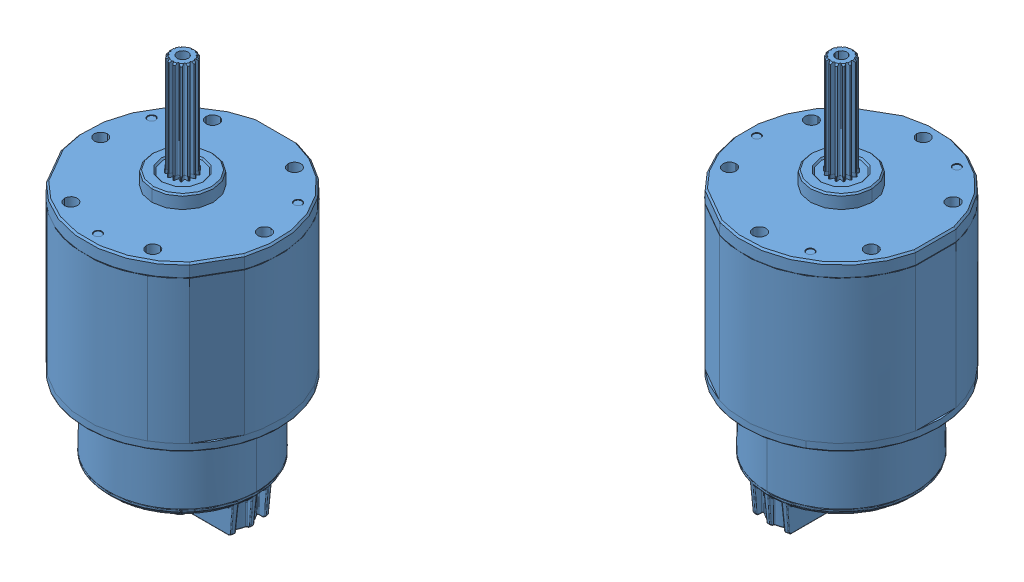
SolidWorks assembly MK4Motors, configuration Default. Lengths in mm.
Overall size (162.75 116.08 164.3).
2 component instances, 1 part files, 0 mates.
Components (placement in the parent):
- Motor, Falcon500.STEP-1: Motor, Falcon500.STEP [Default] at (-158.75 82.1244 -56.515) x (0 0 1) z (0 1 0) size (61.56 60.51 116.08)
- Motor, Falcon500.STEP-2: Motor, Falcon500.STEP [Default] at (-56.515 82.1244 -158.75) x (-1 0 0) z (0 1 0) size (61.56 60.51 116.08)
